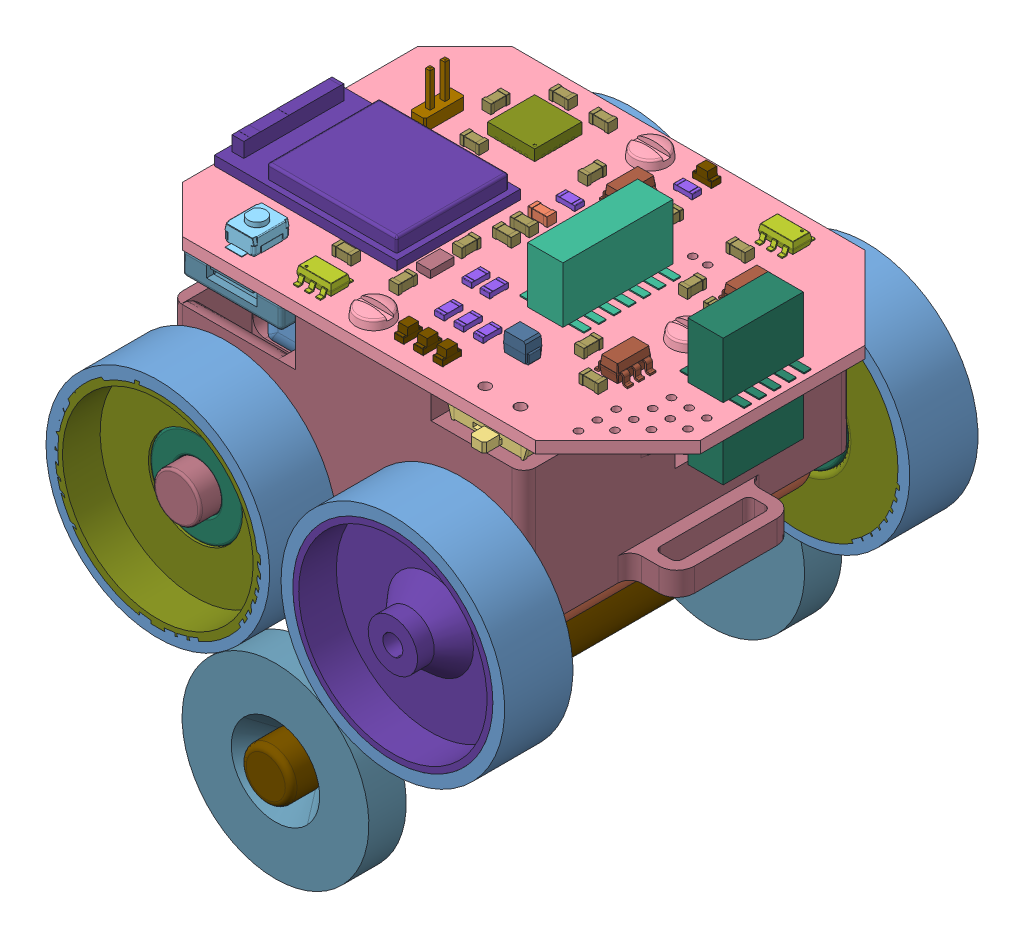
SolidWorks assembly AstroAnt_small_magnet, configuration Default. Lengths in mm.
Overall size (43.22 45.41 41.85).
154 component instances, 38 part files, 26 mates.
Components (placement in the parent):
- LiPo_360mAh-1: LiPo_360mAh [Default] at (6.8166 4.9998 44.2756) size (25 7 18)
- PA2-50-1: PA2-50 [Default] at (8.0673 -18.301 41.8029) x (0 0 1) z (0.952879 0.303349 0) size (29.1 8 8)
- PA2-50-2: PA2-50 [Default] at (-4.1563 19.5334 49.6029) x (0 0 -1) z (0.755989 -0.654584 0) size (29.1 8 8)
- 92120A150_Brass Heat-Set Inserts for Plastic-1: 92120A150_Brass Heat-Set Inserts for Plastic [92120A150] at (19.9543 12.4998 45.7029) size (2.56 3.33 2.56)
- 92120A150_Brass Heat-Set Inserts for Plastic-2: 92120A150_Brass Heat-Set Inserts for Plastic [92120A150] at (4.9543 12.4998 33.9529) size (2.56 3.33 2.56)
- 92120A150_Brass Heat-Set Inserts for Plastic-3: 92120A150_Brass Heat-Set Inserts for Plastic [92120A150] at (4.9543 12.4998 57.4529) size (2.56 3.33 2.56)
- 91460A005_METRIC CHEESE HEAD SLOTTED MACHINE SCREW-8: 91460A005_METRIC CHEESE HEAD SLOTTED MACHINE SCREW [91460A005] at (4.9543 14.9998 57.4529) x (1 0 0) z (0 1 0) size (3 3 7.1)
- 91460A005_METRIC CHEESE HEAD SLOTTED MACHINE SCREW-9: 91460A005_METRIC CHEESE HEAD SLOTTED MACHINE SCREW [91460A005] at (4.9543 14.9998 33.9529) x (1 0 0) z (0 1 0) size (3 3 7.1)
- 91460A005_METRIC CHEESE HEAD SLOTTED MACHINE SCREW-10: 91460A005_METRIC CHEESE HEAD SLOTTED MACHINE SCREW [91460A005] at (19.9543 14.9998 45.7029) x (1 0 0) z (0 1 0) size (3 3 7.1)
- 92120A150_Brass Heat-Set Inserts for Plastic-4: 92120A150_Brass Heat-Set Inserts for Plastic [92120A150] at (4.9543 1.4998 57.4529) x (-0.616962 0 -0.786993) z (0.786993 0 -0.616962) size (2.56 3.33 2.56)
- 92120A150_Brass Heat-Set Inserts for Plastic-5: 92120A150_Brass Heat-Set Inserts for Plastic [92120A150] at (4.9543 1.4998 33.9529) x (-0.616962 0 -0.786993) z (0.786993 0 -0.616962) size (2.56 3.33 2.56)
- 91460A005_METRIC CHEESE HEAD SLOTTED MACHINE SCREW-14: 91460A005_METRIC CHEESE HEAD SLOTTED MACHINE SCREW [91460A005] at (4.9543 -2.5002 57.4529) x (0.663599 0 0.748089) z (0 -1 0) size (3 3 7.1)
- 91460A005_METRIC CHEESE HEAD SLOTTED MACHINE SCREW-15: 91460A005_METRIC CHEESE HEAD SLOTTED MACHINE SCREW [91460A005] at (4.9543 -2.5002 33.9529) x (0.663599 0 0.748089) z (0 -1 0) size (3 3 7.1)
- mainboard_v1.step-1: mainboard_v1.step [Default] at (-103.0457 13.9998 235.7029) x (0 0 -1) z (0 1 0) size (29.41 41 10.8)
  - B3U-1000P.step-1: B3U-1000P.step [Default] at (178.95 -97.38 1.05) x (1 0 0) z (0 -1 0) size (4 1.75 2.5)
    - COMPOUND.step-1: COMPOUND.step [Default] at origin size (4 1.75 2.5)
  - 20021321-00014C1LF.step-1: 20021321-00014C1LF.step [Default] at (190 -115.5 1.05) size (9.35 5.45 4.85)
    - COMPOUND-0.step-1: COMPOUND-0.step [Default] at origin size (9.35 5.45 4.85)
  - MP6513GJ-Z.step-1: MP6513GJ-Z.step [Default] at (201.21 -120 1.05) x (-1 0 0) z (0 0 1) size (2.8 2.9 1)
    - COMPOUND-1.step-1: COMPOUND-1.step [Default] at origin size (2.8 2.9 1)
  - MP6513GJ-Z.step-2: MP6513GJ-Z.step [Default] at (178.51 -103.46 1.05) size (2.8 2.9 1)
    - COMPOUND-1.step-1: COMPOUND-1.step [Default] at origin size (2.8 2.9 1)
  - R_0603_1608Metric.step-1: R_0603_1608Metric.step [Default] at (195.55 -104.38 -0.05) x (1 0 0) z (0 0 -1) size (1.6 0.8 0.45)
    - SOLID.step-1: SOLID.step [Default] at origin size (1.6 0.8 0.45)
  - R_0603_1608Metric.step-2: R_0603_1608Metric.step [Default] at (192.6 -99.86 -0.05) x (0 1 0) z (0 0 -1) size (1.6 0.8 0.45)
    - SOLID.step-1: SOLID.step [Default] at origin size (1.6 0.8 0.45)
  - PinHeader_2x01_P1.27mm_Vertical.step-1: PinHeader_2x01_P1.27mm_Vertical.step [Default] at (194.96 -96.07 1.05) size (3.4 1.27 6.3)
    - SOLID-2.step-1: SOLID-2.step [Default] at origin size (3.4 1.27 6.3)
  - TAJP106K010RNJ.step-1: TAJP106K010RNJ.step [Default] at (196.22 -98.14 -0.05) x (-1 0 0) z (0 0 -1) size (2.05 1.4 1.7)
    - COMPOUND-3.step-1: COMPOUND-3.step [Default] at origin size (2.05 1.4 1.7)
  - TAJP106K010RNJ.step-2: TAJP106K010RNJ.step [Default] at (181.68 -117.23 1.05) x (0 1 0) z (0 0 1) size (2.05 1.4 1.7)
    - COMPOUND-3.step-1: COMPOUND-3.step [Default] at origin size (2.05 1.4 1.7)
  - SOT-23-5.step-1: SOT-23-5.step [Default] at (195.38 -122.78 1.05) x (0 1 0) z (0 0 1) size (2.8 2.9 1.55)
    - SOLID-4.step-1: SOLID-4.step [Default] at origin size (2.8 2.9 1.55)
  - C_0603_1608Metric.step-1: C_0603_1608Metric.step [Default] at (192.91 -122.55 1.05) x (0 -1 0) z (0 0 1) size (1.6 0.8 0.8)
    - SOLID-5.step-1: SOLID-5.step [Default] at origin size (1.6 0.8 0.8)
  - C_0603_1608Metric.step-2: C_0603_1608Metric.step [Default] at (193.57 -119.76 1.05) size (1.6 0.8 0.8)
    - SOLID-5.step-1: SOLID-5.step [Default] at origin size (1.6 0.8 0.8)
  - ECS-.327-12.5-12-TR.step-1: ECS-.327-12.5-12-TR.step [Default] at (184.31 -107.18 1.05) size (2 1.2 0.7)
    - COMPOUND-6.step-1: COMPOUND-6.step [Default] at origin size (2 1.2 0.7)
  - C_0603_1608Metric.step-3: C_0603_1608Metric.step [Default] at (197.67 -113.69 1.05) size (1.6 0.8 0.8)
    - SOLID-5.step-1: SOLID-5.step [Default] at origin size (1.6 0.8 0.8)
  - C_0603_1608Metric.step-4: C_0603_1608Metric.step [Default] at (197.64 -107.18 1.05) size (1.6 0.8 0.8)
    - SOLID-5.step-1: SOLID-5.step [Default] at origin size (1.6 0.8 0.8)
  - C_0603_1608Metric.step-5: C_0603_1608Metric.step [Default] at (190.96 -108.09 1.05) x (0 1 0) z (0 0 1) size (1.6 0.8 0.8)
    - SOLID-5.step-1: SOLID-5.step [Default] at origin size (1.6 0.8 0.8)
  - 1734592-6.step-1: 1734592-6.step [Default] at (203.79 -118 -1.05) x (0 -1 0) z (1 0 0) size (8.43 2.05 5.11)
    - SOLID-7.step-1: SOLID-7.step [Default] at origin size (8.43 2.05 5.11)
  - 1734592-6.step-2: 1734592-6.step [Default] at (176.19 -98 -1.05) x (0 1 0) z (-1 0 0) size (8.43 2.05 5.11)
    - SOLID-7.step-1: SOLID-7.step [Default] at origin size (8.43 2.05 5.11)
  - 20021321-00010C4LF.step-1: 20021321-00010C4LF.step [Default] at (190 -127.85 -0.05) x (1 0 0) z (0 0 -1) size (6.81 5.45 4.85)
    - COMPOUND-8.step-1: COMPOUND-8.step [Default] at origin size (6.81 5.45 4.85)
  - 20021321-00010C4LF.step-2: 20021321-00010C4LF.step [Default] at (190 -127.85 1.05) size (6.81 5.45 4.85)
    - COMPOUND-8.step-1: COMPOUND-8.step [Default] at origin size (6.81 5.45 4.85)
  - C_0603_1608Metric.step-6: C_0603_1608Metric.step [Default] at (181.31 -102.6 1.05) x (0 -1 0) z (0 0 1) size (1.6 0.8 0.8)
    - SOLID-5.step-1: SOLID-5.step [Default] at origin size (1.6 0.8 0.8)
  - C_0603_1608Metric.step-7: C_0603_1608Metric.step [Default] at (198.25 -119.14 1.05) x (0 -1 0) z (0 0 1) size (1.6 0.8 0.8)
    - SOLID-5.step-1: SOLID-5.step [Default] at origin size (1.6 0.8 0.8)
  - MPU6050.step-1: MPU6050.step [Default] at (198.43 -101.5 1.05) x (0 1 0) z (1 0 0) size (4 0.95 4)
    - COMPOUND-9.step-1: COMPOUND-9.step [Default] at origin size (4 0.95 4)
  - C_0603_1608Metric.step-8: C_0603_1608Metric.step [Default] at (194.9 -99.89 1.05) x (0 -1 0) z (0 0 1) size (1.6 0.8 0.8)
    - SOLID-5.step-1: SOLID-5.step [Default] at origin size (1.6 0.8 0.8)
  - C_0603_1608Metric.step-9: C_0603_1608Metric.step [Default] at (201.98 -100.38 1.05) x (0 -1 0) z (0 0 1) size (1.6 0.8 0.8)
    - SOLID-5.step-1: SOLID-5.step [Default] at origin size (1.6 0.8 0.8)
  - C_0603_1608Metric.step-10: C_0603_1608Metric.step [Default] at (201.98 -103.78 1.05) x (0 1 0) z (0 0 1) size (1.6 0.8 0.8)
    - SOLID-5.step-1: SOLID-5.step [Default] at origin size (1.6 0.8 0.8)
  - C_0603_1608Metric.step-11: C_0603_1608Metric.step [Default] at (198.81 -97.82 1.05) size (1.6 0.8 0.8)
    - SOLID-5.step-1: SOLID-5.step [Default] at origin size (1.6 0.8 0.8)
  - SOT-23-5.step-2: SOT-23-5.step [Default] at (184.86 -122.77 1.05) x (0 1 0) z (0 0 1) size (2.8 2.9 1.55)
    - SOLID-4.step-1: SOLID-4.step [Default] at origin size (2.8 2.9 1.55)
  - SOT-23-5.step-3: SOT-23-5.step [Default] at (197.58 -110.46 1.05) x (0 1 0) z (0 0 1) size (2.8 2.9 1.55)
    - SOLID-4.step-1: SOLID-4.step [Default] at origin size (2.8 2.9 1.55)
  - MDBT50Q-1MV2.step-1: MDBT50Q-1MV2.step [Default] at (187.3136 -98.605 1.0754) x (-1 0 0) z (0 1 0) size (10.5 2.06 15.5)
    - SOLID-10.step-1: SOLID-10.step [Default] at origin size (10.5 2.06 15.5)
  - C_0603_1608Metric.step-12: C_0603_1608Metric.step [Default] at (189.44 -108.09 1.05) x (0 1 0) z (0 0 1) size (1.6 0.8 0.8)
    - SOLID-5.step-1: SOLID-5.step [Default] at origin size (1.6 0.8 0.8)
  - C_0603_1608Metric.step-13: C_0603_1608Metric.step [Default] at (181.57 -107.18 1.05) x (-1 0 0) z (0 0 1) size (1.6 0.8 0.8)
    - SOLID-5.step-1: SOLID-5.step [Default] at origin size (1.6 0.8 0.8)
  - C_0603_1608Metric.step-14: C_0603_1608Metric.step [Default] at (186.97 -107.18 1.05) size (1.6 0.8 0.8)
    - SOLID-5.step-1: SOLID-5.step [Default] at origin size (1.6 0.8 0.8)
  - C_0603_1608Metric.step-15: C_0603_1608Metric.step [Default] at (184.77 -119.75 1.05) x (-1 0 0) z (0 0 1) size (1.6 0.8 0.8)
    - SOLID-5.step-1: SOLID-5.step [Default] at origin size (1.6 0.8 0.8)
  - C_0603_1608Metric.step-16: C_0603_1608Metric.step [Default] at (182.37 -122.54 1.05) x (0 -1 0) z (0 0 1) size (1.6 0.8 0.8)
    - SOLID-5.step-1: SOLID-5.step [Default] at origin size (1.6 0.8 0.8)
  - LED_0603_1608Metric.step-1: LED_0603_1608Metric.step [Default] at (178.19 -111.01 1.05) size (1.6 0.8 1.1)
    - SOLID-11.step-1: SOLID-11.step [Default] at origin size (1.6 0.8 1.1)
  - LED_0603_1608Metric.step-2: LED_0603_1608Metric.step [Default] at (178.19 -112.66 1.05) size (1.6 0.8 1.1)
    - SOLID-11.step-1: SOLID-11.step [Default] at origin size (1.6 0.8 1.1)
  - LED_0603_1608Metric.step-3: LED_0603_1608Metric.step [Default] at (178.19 -114.31 1.05) size (1.6 0.8 1.1)
    - SOLID-11.step-1: SOLID-11.step [Default] at origin size (1.6 0.8 1.1)
  - LED_0603_1608Metric.step-4: LED_0603_1608Metric.step [Default] at (202.34 -112.21 1.05) x (0 1 0) z (0 0 1) size (1.6 0.8 1.1)
    - SOLID-11.step-1: SOLID-11.step [Default] at origin size (1.6 0.8 1.1)
  - 473460001.step-1: 473460001.step [Default] at (201.68 -99.72 -1.25) x (0 -1 0) z (1 0 0) size (7.98 2.94 5.43)
    - COMPOUND-12.step-1: COMPOUND-12.step [Default] at origin size (7.98 2.94 5.43)
  - L_0603_1608Metric.step-1: L_0603_1608Metric.step [Default] at (192.48 -108.09 1.05) x (0 1 0) z (0 0 1) size (1.6 0.8 0.8)
    - SOLID-13.step-1: SOLID-13.step [Default] at origin size (1.6 0.8 0.8)
  - R_0603_1608Metric.step-3: R_0603_1608Metric.step [Default] at (185.18 -111.31 1.05) x (-1 0 0) z (0 0 1) size (1.6 0.8 0.45)
    - SOLID.step-1: SOLID.step [Default] at origin size (1.6 0.8 0.45)
  - R_0603_1608Metric.step-4: R_0603_1608Metric.step [Default] at (185.18 -109.77 1.05) size (1.6 0.8 0.45)
    - SOLID.step-1: SOLID.step [Default] at origin size (1.6 0.8 0.45)
  - R_0603_1608Metric.step-5: R_0603_1608Metric.step [Default] at (181.62 -111.01 1.05) size (1.6 0.8 0.45)
    - SOLID.step-1: SOLID.step [Default] at origin size (1.6 0.8 0.45)
  - R_0603_1608Metric.step-6: R_0603_1608Metric.step [Default] at (181.62 -112.66 1.05) size (1.6 0.8 0.45)
    - SOLID.step-1: SOLID.step [Default] at origin size (1.6 0.8 0.45)
  - R_0603_1608Metric.step-7: R_0603_1608Metric.step [Default] at (181.62 -114.31 1.05) x (-1 0 0) z (0 0 1) size (1.6 0.8 0.45)
    - SOLID.step-1: SOLID.step [Default] at origin size (1.6 0.8 0.45)
  - R_0603_1608Metric.step-8: R_0603_1608Metric.step [Default] at (194.84 -108.1 1.05) x (0 1 0) z (0 0 1) size (1.6 0.8 0.45)
    - SOLID.step-1: SOLID.step [Default] at origin size (1.6 0.8 0.45)
  - R_0603_1608Metric.step-9: R_0603_1608Metric.step [Default] at (200.69 -112.2325 1.05) x (0 1 0) z (0 0 1) size (1.6 0.8 0.45)
    - SOLID.step-1: SOLID.step [Default] at origin size (1.6 0.8 0.45)
  - R_0603_1608Metric.step-10: R_0603_1608Metric.step [Default] at (196.22 -101.51 -0.05) x (-1 0 0) z (0 0 -1) size (1.6 0.8 0.45)
    - SOLID.step-1: SOLID.step [Default] at origin size (1.6 0.8 0.45)
  - R_0603_1608Metric.step-11: R_0603_1608Metric.step [Default] at (196.22 -99.9725 -0.05) x (-1 0 0) z (0 0 -1) size (1.6 0.8 0.45)
    - SOLID.step-1: SOLID.step [Default] at origin size (1.6 0.8 0.45)
  - SW_SPDT_PCM12.step-1: SW_SPDT_PCM12.step [Default] at (178.18 -119.37 -0.05) x (0 1 0) z (0 0 -1) size (7.7 5 2)
    - SOLID-14.step-1: SOLID-14.step [Default] at origin size (7.7 5 2)
  - COMPOUND-15.step-1: COMPOUND-15.step [Default] at origin size (28 41 1)
- 91613A020_METRIC CHEESE HEAD SLOTTED MACHINE SCREW-1: 91613A020_METRIC CHEESE HEAD SLOTTED MACHINE SCREW [91613A020] at (1.2533 -0.5002 54.4029) x (1 0 0) z (0 1 0) size (3 3 5.08)
- 91613A020_METRIC CHEESE HEAD SLOTTED MACHINE SCREW-2: 91613A020_METRIC CHEESE HEAD SLOTTED MACHINE SCREW [91613A020] at (8.6533 -0.5002 54.4029) x (1 0 0) z (0 1 0) size (3 3 5.08)
- 91613A020_METRIC CHEESE HEAD SLOTTED MACHINE SCREW-3: 91613A020_METRIC CHEESE HEAD SLOTTED MACHINE SCREW [91613A020] at (1.2533 -0.5002 37.0029) x (1 0 0) z (0 1 0) size (3 3 5.08)
- IR_TEMP_V2.step-3: IR_TEMP_V2.step [Default] at (118.9553 -0.5002 109.7029) x (-1 0 0) z (0 1 0) size (10 20 4.8)
  - Board_Geoms_380f.step-1: Board_Geoms_380f.step [Default] at origin size (10 20 1.11)
    - Pcb_380f.step-1: Pcb_380f.step [Default] at origin size (10 20 1)
    - topTracks_380f.step-1: topTracks_380f.step [Default] at (0 0 0.01) size (9.62 17.53 0.05)
    - botTracks_380f.step-1: botTracks_380f.step [Default] at (0 0 -1.01) size (9.25 16.88 0.05)
  - Step_Models_380f.step-1: Step_Models_380f.step [Default] at origin size (9.46 10.17 4.8)
    - Top_380f.step-1: Top_380f.step [Default] at origin size (9.46 10.17 1.2)
      - IC1_PW14_613E6C6D.step-1: IC1_PW14_613E6C6D.step [Default] at (113.99 -59.48 0) x (-1 0 0) z (0 1 0) size (6.4 1.2 5)
      - C1_C_0402_1005Metric_613EDDF6.step-1: C1_C_0402_1005Metric_613EDDF6.step [Default] at (110.5 -64.26 0) x (-1 0 0) z (0 0 1) size (1 0.5 0.5)
      - C1_C_0402_1005Metric_613EDDF6.step-2: C1_C_0402_1005Metric_613EDDF6.step [Default] at (109.52 -61.07 0) x (0 -1 0) z (0 0 1) size (1 0.5 0.5)
      - C1_C_0402_1005Metric_613EDDF6.step-3: C1_C_0402_1005Metric_613EDDF6.step [Default] at (118.48 -60.86 0) x (0 -1 0) z (0 0 1) size (1 0.5 0.5)
      - C1_C_0402_1005Metric_613EDDF6.step-4: C1_C_0402_1005Metric_613EDDF6.step [Default] at (118.48 -58.59 0) x (0 -1 0) z (0 0 1) size (1 0.5 0.5)
      - C1_C_0402_1005Metric_613EDDF6.step-5: C1_C_0402_1005Metric_613EDDF6.step [Default] at (113.32 -66.9 0) size (1 0.5 0.5)
      - R1_R_0402_1005Metric_613EDE7A.step-1: R1_R_0402_1005Metric_613EDE7A.step [Default] at (110.98 -63.1 0) size (1 0.5 0.35)
      - R1_R_0402_1005Metric_613EDE7A.step-2: R1_R_0402_1005Metric_613EDE7A.step [Default] at (111.68 -66.3 0) x (0 1 0) z (0 0 1) size (1 0.5 0.35)
    - Bot_380f.step-1: Bot_380f.step [Default] at origin size (6.35 7.64 4.6)
      - U1_ZTP-135SR_613E6CD4.step-1: U1_ZTP-135SR_613E6CD4.step [Default] at (114 -64 -1) x (-1 0 0) z (0 -1 0) size (6.35 4.6 5.4)
      - C1_C_0402_1005Metric_613EDDF6.step-1: C1_C_0402_1005Metric_613EDDF6.step [Default] at (115.07 -59.56 -1) x (0 -1 0) z (0 0 -1) size (1 0.5 0.5)
      - R1_R_0402_1005Metric_613EDE7A.step-1: R1_R_0402_1005Metric_613EDE7A.step [Default] at (113.64 -59.58 -1) x (0 -1 0) z (0 0 -1) size (1 0.5 0.35)
- Body_simple-1: Body_simple [Default] at (4.8007 -0.0002 38.7677) size (34 16 37)
- RA22CS-N.step-5: RA22CS-N.step [Default] at (4.9543 -14.2854 27.1904) x (0.988519 -0.1511 0) z (0.1511 0.988519 0) size (15.88 3.17 15.88)
- ball_bearing_5x11x4mm-1: ball_bearing_5x11x4mm [Default] at (-45.4624 -2.1758 28.9029) x (0.999925 -0.012245 0) z (0 0 1) size (8 8 2.5)
- wheel_holder_non_motor-1: wheel_holder_non_motor [Default] at (-70.2522 1.7638 25.6029) size (17.5 17.5 5.8)
- wheel_holder_non_motor-2: wheel_holder_non_motor [Default] at (-19.1131 -84.0559 65.8029) x (0.185441 0.982655 0) z (0 0 -1) size (17.5 17.5 5.8)
- ball_bearing_5x11x4mm-2: ball_bearing_5x11x4mm [Default] at (-30.2803 -54.9376 62.5029) x (0.373101 0.927791 0) z (0 0 -1) size (8 8 2.5)
- wheel_motor-1: wheel_motor [Default] at (24.0366 1.7037 25.5779) size (17 17 5.8)
- wheel_motor-2: wheel_motor [Default] at (15.5431 29.126 65.8279) x (-0.038296 0.999266 0) z (0 0 -1) size (17 17 5.8)
- RA22CS-N.step-8: RA22CS-N.step [Default] at (4.9543 -14.2854 64.2154) x (-0.693236 -0.720711 0) z (-0.720711 0.693236 0) size (15.88 3.17 15.88)
- magnet_wheel_holder-1: magnet_wheel_holder [Default] at (28.927 -0.7064 28.7779) size (6 6 41.85)
- tire-1: tire [Default] at (38.167 -1.442 25.5779) size (19 19 5.8)
- tire-2: tire [Default] at (58.167 -1.442 25.6029) size (19 19 5.8)
- tire-3: tire [Default] at (38.167 -1.442 60.0029) size (19 19 5.8)
- tire-4: tire [Default] at (58.167 -1.442 60.0279) size (19 19 5.8)
- motor_holder-2: motor_holder [Default] at (-0.192 -4.5002 11.9282) size (20 4.13 28)
Mates (geometry in assembly coordinates):
- Coincident100: coincident anti-aligned: plane of mainboard_v1.step-1/COMPOUND-15.step-1 through (6.7692 13.9998 45.7029) normal (0 -1 0); plane of Body_simple-1 through (4.8007 13.9998 38.7677) normal (0 1 0)
- Concentric58: concentric anti-aligned: cylinder of PA2-50-2 through (-5.0457 -0.0002 33.4029) axis (0 0 1) radius 4; cylinder of Body_simple-1 through (-5.0457 -0.0002 57.7029) axis (0 0 -1) radius 4.1
- Concentric59: concentric aligned: cylinder of mainboard_v1.step-1/COMPOUND-15.step-1 through (19.9543 13.4998 45.7029) axis (0 1 0) radius 0.85; cylinder of Body_simple-1 through (19.9543 5.9998 45.7029) axis (0 1 0) radius 1.15
- Concentric63: concentric anti-aligned: cylinder of ball_bearing_5x11x4mm-1 through (14.9543 -0.0002 31.4029) axis (0 0 -1) radius 4; cylinder of wheel_holder_non_motor-1 through (14.9543 -0.0002 25.6029) axis (0 0 1) radius 4
- Concentric66: concentric anti-aligned: cylinder of Body_simple-1 through (14.9543 -0.0002 27.2029) axis (0 0 1) radius 2; cylinder of ball_bearing_5x11x4mm-1 through (14.9543 -0.0002 32.9029) axis (0 0 -1) radius 2
- Distance2: distance = 0.3 mm anti-aligned: plane of wheel_holder_non_motor-1 through (14.9543 -0.0002 31.4029) normal (0 0 1); plane of Body_simple-1 through (-10.0457 13.9998 31.7029) normal (0 0 -1)
- Coincident105: coincident aligned: plane of ball_bearing_5x11x4mm-1 through (14.9543 -0.0002 31.4029) normal (0 0 1); plane of wheel_holder_non_motor-1 through (14.9543 -0.0002 31.4029) normal (0 0 1)
- Distance3: distance = 0.3 mm anti-aligned: plane of wheel_holder_non_motor-2 through (-5.0457 -0.0002 60.0029) normal (0 0 -1); plane of Body_simple-1 through (-10.0457 13.9998 59.7029) normal (0 0 1)
- Concentric67: concentric aligned: cylinder of Body_simple-1 through (-5.0457 -0.0002 64.2029) axis (0 0 -1) radius 2; cylinder of wheel_holder_non_motor-2 through (-5.0457 -0.0002 65.8029) axis (0 0 -1) radius 4
- Coincident107: coincident aligned: plane of wheel_holder_non_motor-2 through (-5.0457 -0.0002 60.0029) normal (0 0 -1); plane of ball_bearing_5x11x4mm-2 through (-5.0457 -0.0002 60.0029) normal (0 0 -1)
- Concentric68: concentric anti-aligned: cylinder of Body_simple-1 through (-5.0457 -0.0002 64.2029) axis (0 0 -1) radius 2; cylinder of ball_bearing_5x11x4mm-2 through (-5.0457 -0.0002 58.5029) axis (0 0 1) radius 2
- Concentric80: concentric anti-aligned: cylinder of RA22CS-N.step-5 through (4.9543 -14.2854 25.6029) axis (0 0 1) radius 7.9375; cylinder of RA22CS-N.step-8 through (4.9543 -14.2854 65.8029) axis (0 0 -1) radius 7.9375
- Concentric82: concentric aligned: cylinder of RA22CS-N.step-5 through (4.9543 -14.2854 27.1904) axis (0 0 1) radius 2.159; cylinder of magnet_wheel_holder-1 through (4.9543 -14.2854 24.7779) axis (0 0 1) radius 2.16
- Coincident122: coincident anti-aligned: plane of RA22CS-N.step-8 through (4.9543 -14.2854 62.6279) normal (0 0 -1); plane of magnet_wheel_holder-1 through (4.9543 -14.2854 62.6279) normal (0 0 1)
- Concentric83: concentric anti-aligned: cylinder of wheel_motor-1 through (-5.0457 -0.0002 31.3779) axis (0 0 -1) radius 8.5; cylinder of tire-1 through (-5.0457 -0.0002 25.5779) axis (0 0 1) radius 8.5
- Coincident123: coincident aligned: plane of wheel_motor-1 through (-5.0457 -0.0002 25.5779) normal (0 0 -1); plane of tire-1 through (-5.0457 -0.0002 25.5779) normal (0 0 -1)
- Concentric84: concentric anti-aligned: cylinder of wheel_holder_non_motor-1 through (14.9543 -0.0002 31.4029) axis (0 0 -1) radius 8.75; cylinder of tire-2 through (14.9543 -0.0002 25.6029) axis (0 0 1) radius 8.5
- Coincident124: coincident aligned: plane of wheel_holder_non_motor-1 through (14.9543 -0.0002 25.6029) normal (0 0 -1); plane of tire-2 through (14.9543 -0.0002 25.6029) normal (0 0 -1)
- Coincident125: coincident aligned: plane of wheel_motor-2 through (14.9543 -0.0002 65.8279) normal (0 0 1); plane of tire-4 through (14.9543 -0.0002 65.8279) normal (0 0 1)
- Concentric85: concentric aligned: cylinder of wheel_motor-2 through (14.9543 -0.0002 60.0279) axis (0 0 1) radius 8.5; cylinder of tire-4 through (14.9543 -0.0002 60.0279) axis (0 0 1) radius 8.5
- Coincident126: coincident aligned: plane of wheel_holder_non_motor-2 through (-5.0457 -0.0002 65.8029) normal (0 0 1); plane of tire-3 through (-5.0457 -0.0002 65.8029) normal (0 0 1)
- Concentric86: concentric aligned: cylinder of wheel_holder_non_motor-2 through (-5.0457 -0.0002 60.0029) axis (0 0 1) radius 8.75; cylinder of tire-3 through (-5.0457 -0.0002 60.0029) axis (0 0 1) radius 8.5
- Concentric94: concentric anti-aligned: cylinder of IR_TEMP_V2.step-3/Step_Models_380f.step-1/Bot_380f.step-1/U1_ZTP-135SR_613E6CD4.step-1 through (4.9553 -4.1002 45.7029) axis (0 1 0) radius 2.35; cylinder of motor_holder-2 through (4.9553 -0.5002 45.7029) axis (0 -1 0) radius 2.5
- Coincident128: coincident anti-aligned: plane of IR_TEMP_V2.step-3/Board_Geoms_380f.step-1/Pcb_380f.step-1 through (4.9553 -1.5002 45.7029) normal (0 -1 0); plane of motor_holder-2 through (-0.192 -1.5002 11.9282) normal (0 1 0)
- Tangent5: tangent anti-aligned: cylinder of RA22CS-N.step-5 through (4.9543 -14.2854 25.6029) axis (0 0 1) radius 7.9375; cylinder of tire-2 through (14.9543 -0.0002 31.4029) axis (0 0 -1) radius 9.5
- Tangent6: tangent anti-aligned: cylinder of RA22CS-N.step-5 through (4.9543 -14.2854 25.6029) axis (0 0 1) radius 7.9375; cylinder of tire-1 through (-5.0457 -0.0002 31.3779) axis (0 0 -1) radius 9.5
